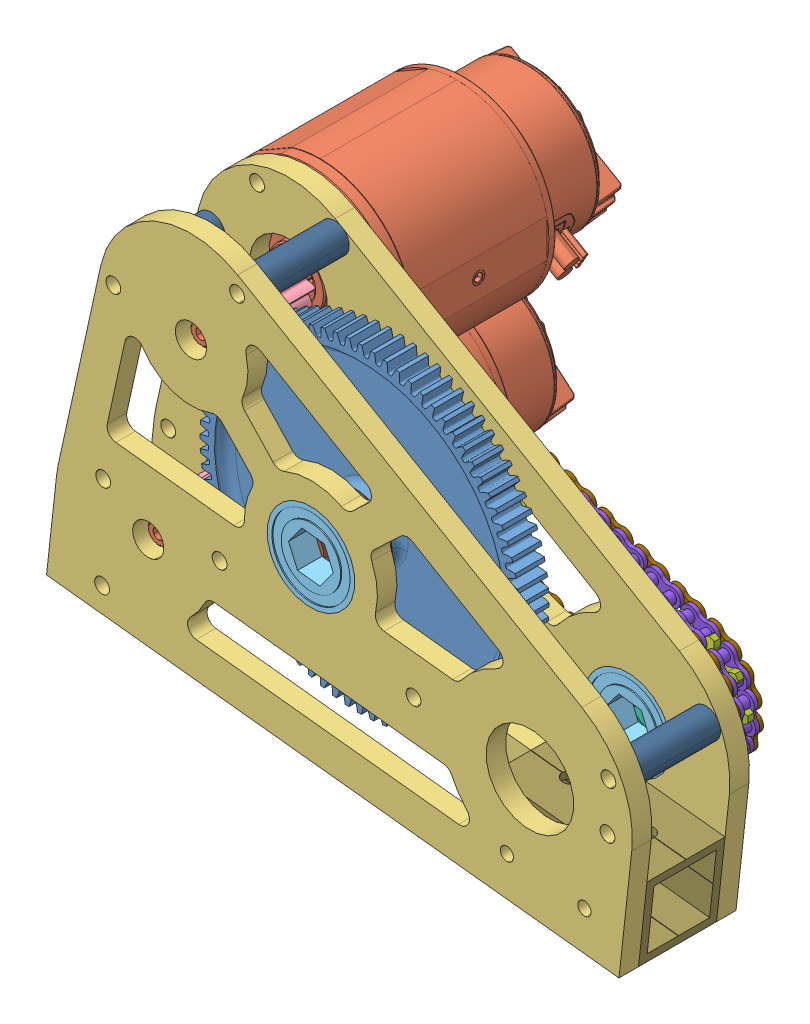
SolidWorks assembly Elevator Gearbox, configuration Default. Lengths in mm.
Overall size (201.77 144.06 120.05).
65 component instances, 12 part files, 48 mates.
Components (placement in the parent):
- 80t Pocketed Gear WCP-1: 80t Pocketed Gear WCP [Default] at (24.0786 56.2628 167.1013) x (-0.980349 0.197269 0) z (0 0 1) size (104.1 104.1 12.6)
- Vexpro - Falcon 500 - 217-6515-1: Vexpro - Falcon 500 - 217-6515 [Default] at (-16.2131 91.7464 112.7507) size (60.01 60.01 116.76)
- Vexpro - Falcon 500 - 217-6515-2: Vexpro - Falcon 500 - 217-6515 [Default] at (-31.2296 28.8555 112.7507) x (0.982938 -0.183935 0) z (0 0 1) size (60.01 60.01 116.76)
- Gearbox Plate 90-1: Gearbox Plate 90 [Default] at (24.0786 56.2628 149.6888) x (0.994032 -0.10909 0) z (0 0 1) size (187.4 124.36 6.35)
- 8t Falcon Pinion-3: 8t Falcon Pinion [Default] at (-28.871 34.7582 163.8513) x (0.826202 0.563374 0) z (0 0 1) size (13.62 13.62 19.05)
- 8t Falcon Pinion-4: 8t Falcon Pinion [Default] at (-14.9805 97.9822 163.8513) x (0.836943 0.54729 0) z (0 0 1) size (13.62 13.62 19.05)
- Vexpro - .5in hex bearing flanged - 217-3875-1: Vexpro - .5in hex bearing flanged - 217-3875 [Default] at (24.0786 56.2628 149.6888) x (0.837594 0.546294 0) z (0.546294 -0.837594 0) size (31.12 7.94 31.12)
- Vexpro - .125 acetal hex spacer - 217-2758-1: Vexpro - .125 acetal hex spacer - 217-2758 [Default] at (24.0786 56.2628 159.2138) size (19.05 19.05 3.17)
- Vexpro - .5in hex bearing flanged - 217-3875-2: Vexpro - .5in hex bearing flanged - 217-3875 [Default] at (95.3405 29.2778 156.0388) x (0.991685 -0.128686 0) z (0.128686 0.991685 0) size (31.12 7.94 31.12)
- 12t sprocket-1: 12t sprocket [Default] at (24.0786 56.2628 137.5159) x (0.762324 0.647195 0) z (0 0 1) size (40.3 40.3 10.67)
- Vexpro - .125 acetal hex spacer - 217-2758-2: Vexpro - .125 acetal hex spacer - 217-2758 [Default] at (24.0786 56.2628 148.1013) x (0.998753 -0.049929 0) z (0 0 1) size (19.05 19.05 3.17)
- 12t sprocket-2: 12t sprocket [Default] at (95.3405 29.2778 136.3983) x (0.93931 0.343069 0) z (0 0 1) size (40.3 40.3 10.67)
- Vexpro - .125 acetal hex spacer - 217-2758-3: Vexpro - .125 acetal hex spacer - 217-2758 [Default] at (95.3405 29.2778 146.5138) x (0.997838 -0.065729 0) z (0 0 1) size (19.05 19.05 3.17)
- Gearbox Chain-1: Gearbox Chain [Default] at (95.3405 29.2778 135.3696) x (0.935195 -0.354134 0) z (0 0 1) size (119.66 43.42 9.52)
  - #25 Roller Chain Inside Link-1: #25 Roller Chain Inside Link [Default] at (17.5785 4.6626 -1.27) x (-0.421188 0.906973 0) z (0 0 1) size (12.24 5.89 5.71)
  - #25 Roller Chain Outside Link-1: #25 Roller Chain Outside Link [Default] at (14.904 10.4219 -2.54) x (-0.707331 0.706882 0) z (0 0 1) size (12.24 5.89 9.53)
  - #25 Roller Chain Outside Link-2: #25 Roller Chain Outside Link [Default] at (18.11 -1.6651 -2.54) x (-0.083697 0.996491 0) z (0 0 1) size (12.24 5.89 9.53)
  - #25 Roller Chain Outside Link-3: #25 Roller Chain Outside Link [Default] at (12.7537 -12.9648 -2.54) x (0.579509 0.814966 0) z (0 0 1) size (12.24 5.89 9.53)
  - #25 Roller Chain Outside Link-4: #25 Roller Chain Outside Link [Default] at (1.3676 -18.1349 -2.54) x (0.968727 0.248131 0) z (0 0 1) size (12.24 5.89 9.53)
  - #25 Roller Chain Outside Link-5: #25 Roller Chain Outside Link [Default] at (-11.3322 -18.1864 -2.54) size (12.24 5.89 9.53)
  - #25 Roller Chain Outside Link-6: #25 Roller Chain Outside Link [Default] at (-24.0322 -18.1864 -2.54) size (12.24 5.89 9.53)
  - #25 Roller Chain Outside Link-7: #25 Roller Chain Outside Link [Default] at (-36.7322 -18.1864 -2.54) size (12.24 5.89 9.53)
  - #25 Roller Chain Outside Link-8: #25 Roller Chain Outside Link [Default] at (-49.4321 -18.1864 -2.54) size (12.24 5.89 9.53)
  - #25 Roller Chain Outside Link-9: #25 Roller Chain Outside Link [Default] at (-62.1321 -18.1864 -2.54) size (12.24 5.89 9.53)
  - #25 Roller Chain Outside Link-10: #25 Roller Chain Outside Link [Default] at (-74.8321 -18.1864 -2.54) size (12.24 5.89 9.53)
  - #25 Roller Chain Outside Link-11: #25 Roller Chain Outside Link [Default] at (-86.8605 -14.7343 -2.54) x (0.900075 -0.435736 0) z (0 0 1) size (12.24 5.89 9.53)
  - #25 Roller Chain Outside Link-12: #25 Roller Chain Outside Link [Default] at (-93.8541 -4.3678 -2.54) x (0.405952 -0.913895 0) z (0 0 1) size (12.24 5.89 9.53)
  - #25 Roller Chain Outside Link-13: #25 Roller Chain Outside Link [Default] at (-92.501 8.0637 -2.54) x (-0.280103 -0.95997 0) z (0 0 1) size (12.24 5.89 9.53)
  - #25 Roller Chain Outside Link-14: #25 Roller Chain Outside Link [Default] at (-83.4408 16.6828 -2.54) x (-0.833726 -0.552178 0) z (0 0 1) size (12.24 5.89 9.53)
  - #25 Roller Chain Outside Link-15: #25 Roller Chain Outside Link [Default] at (-70.914 18.1864 -2.54) x (-0.999988 -0.004905 0) z (0 0 1) size (12.24 5.89 9.53)
  - #25 Roller Chain Outside Link-16: #25 Roller Chain Outside Link [Default] at (-58.214 18.1864 -2.54) x (-1 0 0) z (0 0 1) size (12.24 5.89 9.53)
  - #25 Roller Chain Outside Link-17: #25 Roller Chain Outside Link [Default] at (-45.514 18.1864 -2.54) x (-1 0 0) z (0 0 1) size (12.24 5.89 9.53)
  - #25 Roller Chain Outside Link-18: #25 Roller Chain Outside Link [Default] at (-32.814 18.1864 -2.54) x (-1 0 0) z (0 0 1) size (12.24 5.89 9.53)
  - #25 Roller Chain Outside Link-19: #25 Roller Chain Outside Link [Default] at (-20.1141 18.1864 -2.54) x (-1 0 0) z (0 0 1) size (12.24 5.89 9.53)
  - #25 Roller Chain Outside Link-20: #25 Roller Chain Outside Link [Default] at (-7.4141 18.1864 -2.54) x (-1 0 0) z (0 0 1) size (12.24 5.89 9.53)
  - #25 Roller Chain Outside Link-21: #25 Roller Chain Outside Link [Default] at (5.2389 17.4155 -2.54) x (-0.992603 0.121406 0) z (0 0 1) size (12.24 5.89 9.53)
  - #25 Roller Chain Inside Link-2: #25 Roller Chain Inside Link [Default] at (16.4336 -7.7898 -1.27) x (0.263998 0.964523 0) z (0 0 1) size (12.24 5.89 5.71)
  - #25 Roller Chain Inside Link-3: #25 Roller Chain Inside Link [Default] at (7.519 -16.5593 -1.27) x (0.824369 0.566053 0) z (0 0 1) size (12.24 5.89 5.71)
  - #25 Roller Chain Inside Link-4: #25 Roller Chain Inside Link [Default] at (-4.9822 -18.1864 -1.27) x (0.999967 0.008109 0) z (0 0 1) size (12.24 5.89 5.71)
  - #25 Roller Chain Inside Link-5: #25 Roller Chain Inside Link [Default] at (-17.6822 -18.1864 -1.27) size (12.24 5.89 5.71)
  - #25 Roller Chain Inside Link-6: #25 Roller Chain Inside Link [Default] at (-30.3822 -18.1864 -1.27) size (12.24 5.89 5.71)
  - #25 Roller Chain Inside Link-7: #25 Roller Chain Inside Link [Default] at (-43.0821 -18.1864 -1.27) size (12.24 5.89 5.71)
  - #25 Roller Chain Inside Link-8: #25 Roller Chain Inside Link [Default] at (-55.7821 -18.1864 -1.27) size (12.24 5.89 5.71)
  - #25 Roller Chain Inside Link-9: #25 Roller Chain Inside Link [Default] at (-68.4821 -18.1864 -1.27) size (12.24 5.89 5.71)
  - #25 Roller Chain Inside Link-10: #25 Roller Chain Inside Link [Default] at (-81.145 -17.5012 -1.27) x (0.994161 -0.107906 0) z (0 0 1) size (12.24 5.89 5.71)
  - #25 Roller Chain Inside Link-11: #25 Roller Chain Inside Link [Default] at (-91.2763 -10.171 -1.27) x (0.695403 -0.71862 0) z (0 0 1) size (12.24 5.89 5.71)
  - #25 Roller Chain Inside Link-12: #25 Roller Chain Inside Link [Default] at (-94.2796 1.9679 -1.27) x (0.067009 -0.997752 0) z (0 0 1) size (12.24 5.89 5.71)
  - #25 Roller Chain Inside Link-13: #25 Roller Chain Inside Link [Default] at (-88.735 13.1765 -1.27) x (-0.593066 -0.805154 0) z (0 0 1) size (12.24 5.89 5.71)
  - #25 Roller Chain Inside Link-14: #25 Roller Chain Inside Link [Default] at (-77.2639 18.1553 -1.27) x (-0.972743 -0.231884 0) z (0 0 1) size (12.24 5.89 5.71)
  - #25 Roller Chain Inside Link-15: #25 Roller Chain Inside Link [Default] at (-64.564 18.1864 -1.27) x (-1 0 0) z (0 0 1) size (12.24 5.89 5.71)
  - #25 Roller Chain Inside Link-16: #25 Roller Chain Inside Link [Default] at (-51.864 18.1864 -1.27) x (-1 0 0) z (0 0 1) size (12.24 5.89 5.71)
  - #25 Roller Chain Inside Link-17: #25 Roller Chain Inside Link [Default] at (-39.164 18.1864 -1.27) x (-1 0 0) z (0 0 1) size (12.24 5.89 5.71)
  - #25 Roller Chain Inside Link-18: #25 Roller Chain Inside Link [Default] at (-26.464 18.1864 -1.27) x (-1 0 0) z (0 0 1) size (12.24 5.89 5.71)
  - #25 Roller Chain Inside Link-19: #25 Roller Chain Inside Link [Default] at (-13.7641 18.1864 -1.27) x (-1 0 0) z (0 0 1) size (12.24 5.89 5.71)
  - #25 Roller Chain Inside Link-20: #25 Roller Chain Inside Link [Default] at (-1.0641 18.1864 -1.27) x (-1 0 0) z (0 0 1) size (12.24 5.89 5.71)
  - #25 Roller Chain Inside Link-21: #25 Roller Chain Inside Link [Default] at (10.907 14.5527 -1.27) x (-0.892612 0.450825 0) z (0 0 1) size (12.24 5.89 5.71)
- Gearbox Plate 90-2: Gearbox Plate 90 [Outside] at (24.0786 56.2628 181.4388) x (0.994032 -0.10909 0) z (0 0 1) size (187.4 124.36 6.35)
- 1in spacer-1: 1in spacer [Default] at (-40.2289 100.7531 168.7388) x (0 0 1) z (-0.9849 -0.173126 0) size (25.4 9.5 9.5)
- 1in spacer-2: 1in spacer [Default] at (0.0433 118.4625 168.7388) x (0 0 1) z (-0.9849 -0.173126 0) size (25.4 9.5 9.5)
- 1in spacer-3: 1in spacer [Default] at (-43.8949 14.2779 168.7388) x (0 0 1) z (-0.999698 -0.024559 0) size (25.4 9.5 9.5)
- 1in spacer-5: 1in spacer [Default] at (120.8801 42.0941 168.7388) x (0 0 1) z (-0.999698 -0.024559 0) size (25.4 9.5 9.5)
- Vexpro - .5in hex bearing flanged - 217-3875-3: Vexpro - .5in hex bearing flanged - 217-3875 [Default] at (24.0786 56.2628 187.7888) x (0.99379 -0.111271 0) z (0.111271 0.99379 0) size (31.12 7.94 31.12)
- Clamping Shaft Collar - 1_2 Hex ID (217-2737)-1: Clamping Shaft Collar - 1_2 Hex ID (217-2737) [Default] at (24.0786 56.2628 176.6763) size (25.39 25.4 6.35)
- Gear SUpport Mount-1: Gear SUpport Mount [Default] at (-619.12 82.1338 168.7388) x (0 0 1) z (-0.994032 0.10909 0) size (25.4 25.4 25.4)
- Gear SUpport Mount-2: Gear SUpport Mount [Default] at (-644.3684 84.9047 168.7388) x (0 0 1) z (-0.994032 0.10909 0) size (25.4 25.4 25.4)
Mates (geometry in assembly coordinates):
- Coincident2: coincident aligned: plane of Vexpro - Falcon 500 - 217-6515-1 through (-19.743 89.7333 149.6888) normal (0 0 1); plane of Vexpro - Falcon 500 - 217-6515-2 through (-35.0696 27.526 149.6888) normal (0 0 1)
- Concentric1: concentric anti-aligned: circle of 80t Pocketed Gear WCP-1; circle of Gearbox Plate 90-1
- Coincident3: coincident anti-aligned: plane of Vexpro - Falcon 500 - 217-6515-1 through (-19.743 89.7333 149.6888) normal (0 0 1); plane of Gearbox Plate 90-1 through (-28.8711 34.7582 149.6888) normal (0 0 -1)
- Concentric2: concentric anti-aligned: cylinder of Vexpro - Falcon 500 - 217-6515-1 through (-14.9805 97.9822 145.6888) axis (0 0 -1) radius 30; circle of Gearbox Plate 90-1
- Concentric3: concentric aligned: circle of Vexpro - Falcon 500 - 217-6515-2; circle of Gearbox Plate 90-1
- Concentric4: concentric: cylinder of Vexpro - Falcon 500 - 217-6515-2 through (-28.8711 34.7582 184.4888) axis (0 0 1) radius 1.7272; point of 8t Falcon Pinion-3
- Concentric5: concentric: cylinder of Vexpro - Falcon 500 - 217-6515-1 through (-14.9805 97.9822 184.4888) axis (0 0 1) radius 1.7272; point of 8t Falcon Pinion-4
- Coincident5: coincident anti-aligned: plane of Vexpro - Falcon 500 - 217-6515-1 through (-12.1052 97.1887 154.3263) normal (0 0 1); plane of 8t Falcon Pinion-4 through (-19.2539 104.5172 154.3263) normal (0 0 -1)
- Coincident6: coincident anti-aligned: plane of Vexpro - Falcon 500 - 217-6515-2 through (-26.1908 33.4493 154.3263) normal (0 0 1); plane of 8t Falcon Pinion-3 through (-33.27 41.2094 154.3263) normal (0 0 -1)
- Concentric6: concentric anti-aligned: cylinder of Gearbox Plate 90-1 through (24.0786 56.2628 156.0388) axis (0 0 -1) radius 14.2875; cylinder of Vexpro - .5in hex bearing flanged - 217-3875-1 through (24.0786 56.2628 149.6888) axis (0 0 1) radius 14.2748
- Concentric7: concentric aligned: cylinder of 80t Pocketed Gear WCP-1 through (24.0786 56.2628 173.4013) axis (0 0 -1) radius 8.89; cylinder of Vexpro - .125 acetal hex spacer - 217-2758-1 through (24.0786 56.2628 160.8013) axis (0 0 -1) radius 9.525
- Coincident9: coincident anti-aligned: plane of 80t Pocketed Gear WCP-1 through (24.0786 56.2628 160.8013) normal (0 0 -1); plane of Vexpro - .125 acetal hex spacer - 217-2758-1 through (24.0786 56.2628 160.8013) normal (0 0 1)
- Concentric8: concentric aligned: cylinder of Gearbox Plate 90-1 through (95.3405 29.2778 156.0388) axis (0 0 -1) radius 14.2875; cylinder of Vexpro - .5in hex bearing flanged - 217-3875-2 through (95.3405 29.2778 156.0388) axis (0 0 -1) radius 14.2748
- Coincident10: coincident anti-aligned: plane of Gearbox Plate 90-1 through (-28.8711 34.7582 149.6888) normal (0 0 -1); plane of Vexpro - .5in hex bearing flanged - 217-3875-2 through (110.7686 27.2758 149.6888) normal (0 0 1)
- Concentric9: concentric aligned: circle of Vexpro - .5in hex bearing flanged - 217-3875-1; circle of 12t sprocket-1
- Concentric10: concentric anti-aligned: circle of Vexpro - .5in hex bearing flanged - 217-3875-1; cylinder of Vexpro - .125 acetal hex spacer - 217-2758-2 through (24.0786 56.2628 149.6888) axis (0 0 -1) radius 9.525
- Coincident14: coincident anti-aligned: plane of 12t sprocket-2 through (95.3405 29.2778 144.9263) normal (0 0 1); plane of Vexpro - .125 acetal hex spacer - 217-2758-3 through (95.3405 29.2778 144.9263) normal (0 0 -1)
- Coincident15: coincident anti-aligned: plane of Vexpro - .5in hex bearing flanged - 217-3875-2 through (101.6377 28.4607 148.1013) normal (0 0 -1); plane of Vexpro - .125 acetal hex spacer - 217-2758-3 through (95.3405 29.2778 148.1013) normal (0 0 1)
- Concentric11: concentric aligned: cylinder of 12t sprocket-2 through (95.3405 29.2778 144.9263) axis (0 0 -1) radius 12.7; cylinder of Vexpro - .125 acetal hex spacer - 217-2758-3 through (95.3405 29.2778 148.1013) axis (0 0 -1) radius 9.525
- Concentric12: concentric aligned: circle of Vexpro - .5in hex bearing flanged - 217-3875-2; cylinder of Vexpro - .125 acetal hex spacer - 217-2758-3 through (95.3405 29.2778 148.1013) axis (0 0 -1) radius 9.525
- Concentric13: concentric: cylinder of Vexpro - .5in hex bearing flanged - 217-3875-1 through (24.0786 56.2628 149.6888) axis (0 0 1) radius 15.5575; point of Gearbox Chain-1
- Concentric14: concentric: cylinder of Vexpro - .5in hex bearing flanged - 217-3875-2 through (95.3405 29.2778 156.0388) axis (0 0 -1) radius 15.5575; point of Gearbox Chain-1
- Coincident17: coincident anti-aligned: plane of 12t sprocket-2 through (95.3405 29.2778 138.5446) normal (0 0 1); plane of Gearbox Chain-1/#25 Roller Chain Inside Link-20 through (95.4851 46.1128 138.5446) normal (0 0 -1)
- Concentric15: concentric aligned: circle of Gearbox Plate 90-1; circle of Gearbox Plate 90-2
- Coincident18: coincident aligned: plane of Gearbox Plate 90-1 through (-61.9619 8.2122 156.0388) normal (-0.10909 -0.994032 0); plane of Gearbox Plate 90-2 through (-61.9619 8.2122 187.7888) normal (-0.10909 -0.994032 0)
- Concentric16: concentric aligned: cylinder of Gearbox Plate 90-1 through (-40.2289 100.7531 156.0388) axis (0 0 -1) radius 2.413; cylinder of 1in spacer-1 through (-40.2289 100.7531 181.4388) axis (0 0 -1) radius 4.7498
- Coincident20: coincident anti-aligned: plane of Gearbox Plate 90-2 through (-28.8711 34.7582 181.4388) normal (0 0 -1); plane of 1in spacer-1 through (-40.2289 100.7531 181.4388) normal (0 0 1)
- Coincident21: coincident anti-aligned: plane of Gearbox Plate 90-1 through (-28.8711 34.7582 156.0388) normal (0 0 1); plane of 1in spacer-1 through (-40.2289 100.7531 156.0388) normal (0 0 -1)
- Concentric17: concentric aligned: cylinder of Gearbox Plate 90-1 through (0.0433 118.4625 156.0388) axis (0 0 -1) radius 2.413; cylinder of 1in spacer-2 through (0.0433 118.4625 181.4388) axis (0 0 -1) radius 4.7498
- Coincident22: coincident anti-aligned: plane of Gearbox Plate 90-2 through (-28.8711 34.7582 181.4388) normal (0 0 -1); plane of 1in spacer-2 through (0.0433 118.4625 181.4388) normal (0 0 1)
- Concentric18: concentric aligned: cylinder of Gearbox Plate 90-1 through (-43.8949 14.2779 156.0388) axis (0 0 -1) radius 2.413; cylinder of 1in spacer-3 through (-43.8949 14.2779 181.4388) axis (0 0 -1) radius 4.7498
- Coincident23: coincident anti-aligned: plane of Gearbox Plate 90-2 through (-28.8711 34.7582 181.4388) normal (0 0 -1); plane of 1in spacer-3 through (-43.8949 14.2779 181.4388) normal (0 0 1)
- Concentric19: concentric aligned: cylinder of Gearbox Plate 90-2 through (24.0786 56.2628 187.7888) axis (0 0 -1) radius 14.2875; cylinder of Vexpro - .5in hex bearing flanged - 217-3875-3 through (24.0786 56.2628 187.7888) axis (0 0 -1) radius 14.2748
- Coincident24: coincident anti-aligned: plane of Gearbox Plate 90-2 through (-28.8711 34.7582 181.4388) normal (0 0 -1); plane of Vexpro - .5in hex bearing flanged - 217-3875-3 through (39.5395 54.5317 181.4388) normal (0 0 1)
- Coincident25: coincident anti-aligned: plane of Gearbox Plate 90-1 through (-28.8711 34.7582 156.0388) normal (0 0 1); plane of Vexpro - .5in hex bearing flanged - 217-3875-1 through (37.1095 64.7618 156.0388) normal (0 0 -1)
- Coincident26: coincident anti-aligned: plane of Vexpro - .5in hex bearing flanged - 217-3875-1 through (29.3974 59.7318 157.6263) normal (0 0 1); plane of Vexpro - .125 acetal hex spacer - 217-2758-1 through (24.0786 56.2628 157.6263) normal (0 0 -1)
- Coincident28: coincident anti-aligned: plane of Vexpro - .5in hex bearing flanged - 217-3875-1 through (32.1631 61.5357 149.6888) normal (0 0 -1); plane of Vexpro - .125 acetal hex spacer - 217-2758-2 through (24.0786 56.2628 149.6888) normal (0 0 1)
- Coincident29: coincident anti-aligned: plane of 12t sprocket-1 through (13.8084 68.3601 135.3696) normal (0 0 -1); plane of Gearbox Chain-1/#25 Roller Chain Inside Link-14 through (29.5131 73.6183 135.3696) normal (0 0 1)
- Coincident30: coincident anti-aligned: plane of Vexpro - .5in hex bearing flanged - 217-3875-3 through (30.3892 55.5563 179.8513) normal (0 0 -1); plane of Clamping Shaft Collar - 1_2 Hex ID (217-2737)-1 through (24.0786 56.2628 179.8513) normal (0 0 1)
- Concentric21: concentric aligned: cylinder of Vexpro - .5in hex bearing flanged - 217-3875-3 through (24.0786 56.2628 187.7888) axis (0 0 -1) radius 15.5575; cylinder of Clamping Shaft Collar - 1_2 Hex ID (217-2737)-1 through (24.0786 56.2628 179.8513) axis (0 0 -1) radius 12.7
- Concentric23: concentric anti-aligned: circle of Gearbox Plate 90-2; cylinder of 1in spacer-5 through (120.8801 42.0941 181.4388) axis (0 0 -1) radius 4.7498
- Coincident32: coincident anti-aligned: plane of Gearbox Plate 90-1 through (-28.8711 34.7582 156.0388) normal (0 0 1); plane of 1in spacer-5 through (120.8801 42.0941 156.0388) normal (0 0 -1)
- Coincident33: coincident anti-aligned: plane of Gearbox Plate 90-2 through (-28.8711 34.7582 181.4388) normal (0 0 -1); plane of Gear SUpport Mount-1 through (-1365.3335 151.2507 181.4388) normal (0 0 1)
- Coincident34: coincident aligned: plane of Gearbox Plate 90-1 through (124.3227 -12.2316 156.0388) normal (0.994032 -0.10909 0); plane of Gear SUpport Mount-1 through (125.7081 0.3926 168.7388) normal (0.994032 -0.10909 0)
- Coincident35: coincident aligned: plane of Gearbox Plate 90-1 through (-61.9619 8.2122 156.0388) normal (-0.10909 -0.994032 0); plane of Gear SUpport Mount-1 through (-1365.3335 151.2507 156.0388) normal (-0.10909 -0.994032 0)
- Concentric24: concentric aligned: circle of Gearbox Plate 90-2; cylinder of Gear SUpport Mount-2 through (87.8355 4.549 156.0388) axis (0 0 1) radius 2.0701
- Coincident36: coincident anti-aligned: plane of Gearbox Plate 90-2 through (-28.8711 34.7582 181.4388) normal (0 0 -1); plane of Gear SUpport Mount-2 through (-1390.5819 154.0216 181.4388) normal (0 0 1)
- Coincident37: coincident aligned: plane of Gearbox Plate 90-2 through (-61.9619 8.2122 187.7888) normal (-0.10909 -0.994032 0); plane of Gear SUpport Mount-2 through (-1390.5819 154.0216 156.0388) normal (-0.10909 -0.994032 0)
